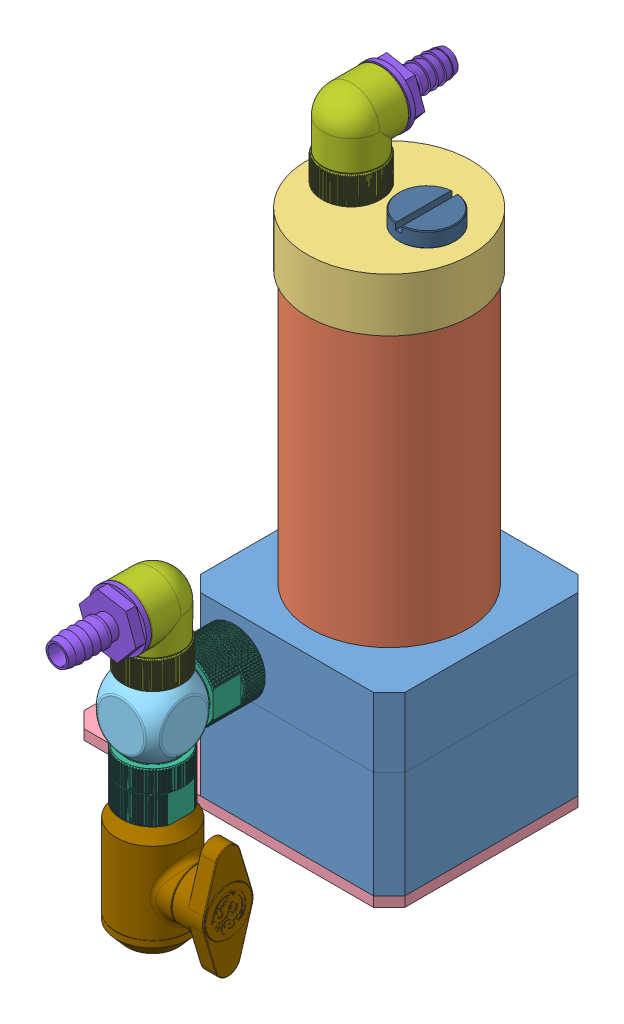
SolidWorks assembly Cooling Pump, configuration Default. Lengths in mm.
Overall size (102 211.26 121.52).
15 component instances, 10 part files, 28 mates.
Components (placement in the parent):
- Freezemod_PU-FS6M-1: Freezemod_PU-FS6M [Default] at origin size (65 159.5 65)
  - Freezemod FS6M_Plus-1: Freezemod FS6M_Plus [Default] at origin size (65 56 65)
  - Freezemod Resevoir-1: Freezemod Resevoir [Default] at (0 99.5 0) x (1 0 0) z (0 1 0) size (52 52 110.5)
    - Innter Tube-1: Innter Tube [Default] at (0 0 99.5) x (1 0 0) z (0 0 -1) size (50 50 100)
    - Top Cap-1: Top Cap [Default] at (0 0 60) x (1 0 0) z (0 0 -1) size (52 52 17)
- Freezemod PU-FS6M Mounting Bracket-1: Freezemod PU-FS6M Mounting Bracket [Default] at (-18.5 0 0) x (0 0 1) z (0 -1 0) size (65 102 3.17)
- Bitspower_T_Fitting-1: Bitspower_T_Fitting [Défaut] at (-16.5 43 58.66) x (0 0 1) z (1 0 0) size (25.4 20.32 25.4)
- EK-AF Extender Rotary M-M G1_4-1: EK-AF Extender Rotary M-M G1_4 [Default] at (-16.5 43 48.5) x (1 0 0) z (0 1 0) size (19.99 25.44 20)
- EK-AF Angled 90deg G1_4-1: EK-AF Angled 90deg G1_4 [Default] at (-16.5 53.66 58.66) x (-1 0 0) z (0 0 -1) size (19 36.31 19.39)
- G14x6mm_Barb-1: G14x6mm_Barb [Défaut] at (-16.5 72.46 73.0225) x (0 0 1) z (-0.923728 -0.383049 0) size (25.52 18.33 18.33)
- EK-AF Extender Rotary M-M G1_4-2: EK-AF Extender Rotary M-M G1_4 [Default] at (-16.5 16.84 58.66) size (19.99 25.44 20)
- G14_Valve-1: G14_Valve [Predeterminado] at (-16.5 -1.16 58.66) x (0 0 -1) z (0 -1 0) size (23 35.7 37.13)
- G14_Plug-1: G14_Plug [Default] at (12 165.3 0) x (1 0 0) z (0 -1 0) size (18.01 18.01 9.94)
- EK-AF Angled 90deg G1_4-3: EK-AF Angled 90deg G1_4 [Default] at (-12 160 0) size (19 36.31 19.39)
- G14x6mm_Barb-2: G14x6mm_Barb [Défaut] at (-12 178.8 -14.3625) x (0 0 -1) z (-0.216826 -0.97621 0) size (25.52 18.33 18.33)
Mates (geometry in assembly coordinates):
- Coincident1: coincident: plane of Freezemod_PU-FS6M-1/Freezemod FS6M_Plus-1 through (0 0 0) normal (0 0 1); plane of assembly through (0 0 0) normal (0 0 1)
- Coincident2: coincident: plane of Freezemod_PU-FS6M-1/Freezemod FS6M_Plus-1 through (0 0 0) normal (0 1 0); plane of assembly through (0 0 0) normal (0 1 0)
- Coincident3: coincident: plane of Freezemod_PU-FS6M-1/Freezemod FS6M_Plus-1 through (0 0 0) normal (1 0 0); plane of assembly through (0 0 0) normal (1 0 0)
- Coincident4: coincident: plane of Freezemod_PU-FS6M-1/Freezemod FS6M_Plus-1 through (0 0 0) normal (0 -1 0); plane of Freezemod PU-FS6M Mounting Bracket-1 through (-18.5 0 0) normal (0 1 0)
- Concentric4: concentric: cylinder of Freezemod_PU-FS6M-1/Freezemod FS6M_Plus-1 through (18.5 0 26.5) axis (0 -1 0) radius 1.65; cylinder of Freezemod PU-FS6M Mounting Bracket-1 through (18.5 -3.175 26.5) axis (0 1 0) radius 2
- Concentric5: concentric: cylinder of Freezemod_PU-FS6M-1/Freezemod FS6M_Plus-1 through (18.5 0 -26.5) axis (0 -1 0) radius 1.65; cylinder of Freezemod PU-FS6M Mounting Bracket-1 through (18.5 -3.175 -26.5) axis (0 1 0) radius 2
- Concentric6: concentric: cylinder of Freezemod_PU-FS6M-1/Freezemod FS6M_Plus-1 through (-16.5 43 12.5) axis (0 0 1) radius 6.5785; cylinder of EK-AF Extender Rotary M-M G1_4-1 through (-16.5 43 42.875) axis (0 0 -1) radius 4.95
- Coincident5: coincident: plane of Freezemod_PU-FS6M-1/Freezemod FS6M_Plus-1 through (-27.5 56 32.5) normal (0 0 1); plane of EK-AF Extender Rotary M-M G1_4-1 through (-24.3 43 32.5) normal (0 0 -1)
- Concentric7: concentric: cylinder of Bitspower_T_Fitting-1 through (-16.5 43 48.5) axis (0 0 -1) radius 5.9436; cylinder of EK-AF Extender Rotary M-M G1_4-1 through (-16.5 43 53) axis (0 0 -1) radius 5.2
- Coincident6: coincident: plane of Bitspower_T_Fitting-1 through (-16.5 43 48.5) normal (0 0 -1); plane of EK-AF Extender Rotary M-M G1_4-1 through (-24.3 43 48.5) normal (0 0 1)
- Parallel2: parallel: plane of Freezemod_PU-FS6M-1/Freezemod FS6M_Plus-1 through (0 0 0) normal (1 0 0); plane of Bitspower_T_Fitting-1 through (-16.5 43 58.66) normal (1 0 0)
- Concentric8: concentric: cylinder of Bitspower_T_Fitting-1 through (-16.5 32.84 58.66) axis (0 -1 0) radius 5.9436; cylinder of EK-AF Angled 90deg G1_4-1 through (-16.5 62.71 58.66) axis (0 -1 0) radius 5.25
- Coincident8: coincident: plane of Bitspower_T_Fitting-1 through (-16.5 53.16 58.66) normal (0 1 0); plane of EK-AF Angled 90deg G1_4-1 through (-8.9 53.16 58.66) normal (0 -1 0)
- Parallel3: parallel: plane of Freezemod_PU-FS6M-1/Freezemod FS6M_Plus-1 through (0 0 0) normal (1 0 0); plane of EK-AF Angled 90deg G1_4-1 through (-16.5 53.66 58.66) normal (-1 0 0)
- Concentric9: concentric: cylinder of EK-AF Angled 90deg G1_4-1 through (-16.5 72.46 68.26) axis (0 0 -1) radius 9; cylinder of G14x6mm_Barb-1 through (-16.5 72.46 73.0225) axis (0 0 -1) radius 1.703
- Coincident10: coincident: plane of EK-AF Angled 90deg G1_4-1 through (-16.5 72.46 68.26) normal (0 0 1); plane of G14x6mm_Barb-1 through (-16.5 72.46 68.26) normal (0 0 -1)
- Concentric10: concentric: cylinder of Bitspower_T_Fitting-1 through (-16.5 32.84 58.66) axis (0 -1 0) radius 5.9436; cylinder of EK-AF Extender Rotary M-M G1_4-2 through (-16.5 22.465 58.66) axis (0 1 0) radius 4.95
- Coincident11: coincident: plane of Bitspower_T_Fitting-1 through (-16.5 32.84 58.66) normal (0 -1 0); plane of EK-AF Extender Rotary M-M G1_4-2 through (-24.3 32.84 58.66) normal (0 1 0)
- Concentric11: concentric: cylinder of EK-AF Extender Rotary M-M G1_4-2 through (-16.5 12.34 58.66) axis (0 1 0) radius 5.2; cylinder of G14_Valve-1 through (-16.5 16.84 58.66) axis (0 1 0) radius 11.5
- Parallel4: parallel: plane of Freezemod_PU-FS6M-1/Freezemod FS6M_Plus-1 through (0 0 0) normal (1 0 0); plane of G14_Valve-1 through (-16.5 -1.16 58.66) normal (1 0 0)
- Coincident13: coincident: plane of EK-AF Extender Rotary M-M G1_4-2 through (-24.3 16.84 58.66) normal (0 -1 0); plane of G14_Valve-1 through (-16.5 16.84 58.66) normal (0 1 0)
- Concentric12: concentric: cylinder of Freezemod_PU-FS6M-1/Freezemod Resevoir-1/Top Cap-1 through (12 159.5 0) axis (0 -1 0) radius 6; cylinder of G14_Plug-1 through (12 155.5 0) axis (0 1 0) radius 5.9
- Tangent1: tangent: plane of Freezemod_PU-FS6M-1/Freezemod Resevoir-1/Top Cap-1 through (0 159.5 0) normal (0 1 0); face of G14_Plug-1
- Coincident14: coincident: plane of Freezemod_PU-FS6M-1/Freezemod Resevoir-1/Top Cap-1 through (0 159.5 0) normal (0 1 0); plane of EK-AF Angled 90deg G1_4-3 through (-19.6 159.5 0) normal (0 -1 0)
- Concentric13: concentric: cylinder of Freezemod_PU-FS6M-1/Freezemod Resevoir-1/Top Cap-1 through (-12 159.5 0) axis (0 -1 0) radius 6; cylinder of EK-AF Angled 90deg G1_4-3 through (-12 169.05 0) axis (0 -1 0) radius 5.25
- Parallel8: parallel: plane of Freezemod_PU-FS6M-1/Freezemod FS6M_Plus-1 through (0 0 0) normal (1 0 0); plane of EK-AF Angled 90deg G1_4-3 through (-12 160 0) normal (1 0 0)
- Concentric14: concentric: cylinder of EK-AF Angled 90deg G1_4-3 through (-12 178.8 -9.6) axis (0 0 1) radius 9; cylinder of G14x6mm_Barb-2 through (-12 178.8 -14.3625) axis (0 0 1) radius 1.703
- Coincident16: coincident: plane of EK-AF Angled 90deg G1_4-3 through (-12 178.8 -9.6) normal (0 0 -1); plane of G14x6mm_Barb-2 through (-12 178.8 -9.6) normal (0 0 1)
